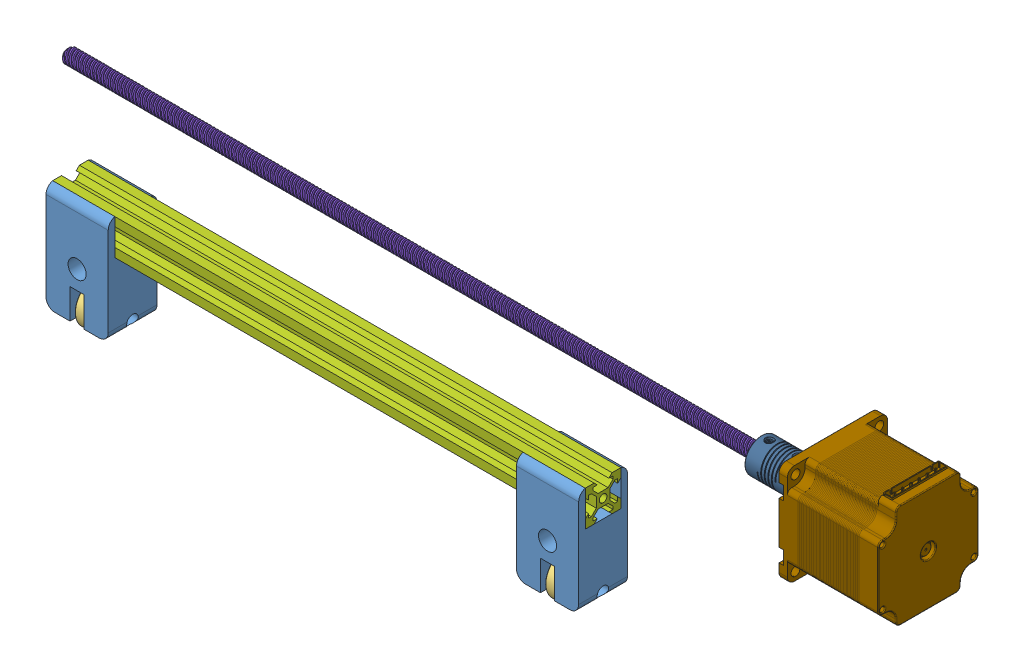
SolidWorks assembly EjeY, configuration Predeterminado. Lengths in mm.
Overall size (487.28 138.63 59).
20 component instances, 10 part files, 8 mates.
Components (placement in the parent):
- SoporteEjeY-1: SoporteEjeY [Predeterminado] at (-17.1016 3.702 20.9937) size (35 68.64 29.7)
  - SujeciónEjeY-1: SujeciónEjeY [Predeterminado] at (-24.012 20.0298 35) size (35 59.86 27.5)
  - T8-Screw-1: T8-Screw [Default] at (-6.512 2.5298 35) x (0 1 0) z (0 0 -1) size (22 22 16.4)
  - skf_bearing_61901_2-1: skf_bearing_61901_2 [Default] at (-9.4581 -20.8302 48.75) x (1 0 0) z (0 -0.067535 0.997717) size (6 24 24)
    - skf_bearing_61901_2_01-1: skf_bearing_61901_2_01 [Default] at origin size (6 24 24)
    - skf_bearing_61901_2_02-1: skf_bearing_61901_2_02 [Default] at origin size (6 16 16)
    - skf_bearing_61901_2_03-1: skf_bearing_61901_2_03 [Default] at origin size (3.18 21.18 20.29)
    - PiezaInterna-1: PiezaInterna [Predeterminado] x (0 0 -1) z (1 0 0) size (12 12 6)
- SoporteEjeY-2: SoporteEjeY [Predeterminado] at (247.6084 3.702 20.9937) size (35 68.64 29.7)
  - SujeciónEjeY-1: SujeciónEjeY [Predeterminado] at (-24.012 20.0298 35) size (35 59.86 27.5)
  - T8-Screw-1: T8-Screw [Default] at (-6.512 2.5298 35) x (0 1 0) z (0 0 -1) size (22 22 16.4)
  - skf_bearing_61901_2-1: skf_bearing_61901_2 [Default] at (-9.4581 -20.8302 48.75) x (1 0 0) z (0 -0.067535 0.997717) size (6 24 24)
    - skf_bearing_61901_2_01-1: skf_bearing_61901_2_01 [Default] at origin size (6 24 24)
    - skf_bearing_61901_2_02-1: skf_bearing_61901_2_02 [Default] at origin size (6 16 16)
    - skf_bearing_61901_2_03-1: skf_bearing_61901_2_03 [Default] at origin size (3.18 21.18 20.29)
    - PiezaInterna-1: PiezaInterna [Predeterminado] x (0 0 -1) z (1 0 0) size (12 12 6)
- BoschEjeY-1: BoschEjeY [Predeterminado] at (-41.1136 18.7318 79.7437) x (0 1 0) z (1 0 0) size (20 20 299.71)
- VarillaEjeY-1: VarillaEjeY [Default] at (339.951 77.517 52.6956) x (0 -1 0) z (1 0 0) size (8.33 8.33 405.47)
- Nema 23-1: Nema 23 [Default] at (424.5988 77.517 52.6956) x (0 0 1) z (-1 0 0) size (56.4 59.4 76.6)
- Coupler 6.35-8mm-1: Coupler 6.35-8mm [Default] at (343.2313 77.517 52.6956) x (0 0 -1) z (1 0 0) size (19.34 19.34 25)
Mates (geometry in assembly coordinates):
- Coincidente1: coincident aligned: plane of SoporteEjeY-1/SujeciónEjeY-1 through (-41.1136 23.7318 59.4937) normal (-1 0 0); plane of BoschEjeY-1 through (-41.1136 18.7318 79.7437) normal (-1 0 0)
- Coincidente2: coincident anti-aligned: plane of SoporteEjeY-1/SujeciónEjeY-1 through (-6.1136 23.7318 79.7437) normal (0 0 -1); plane of BoschEjeY-1 through (258.5964 18.7318 79.7437) normal (0 0 1)
- Coincidente3: coincident anti-aligned: plane of SoporteEjeY-1/SujeciónEjeY-1 through (-6.1136 18.7318 59.7437) normal (0 1 0); plane of BoschEjeY-1 through (258.5964 18.7318 79.7437) normal (0 -1 0)
- Coincidente4: coincident anti-aligned: plane of SoporteEjeY-2/SujeciónEjeY-1 through (258.5964 23.7318 59.7437) normal (0 0 1); plane of BoschEjeY-1 through (258.5964 18.7318 59.7437) normal (0 0 -1)
- Coincidente5: coincident aligned: plane of SoporteEjeY-2/SujeciónEjeY-1 through (258.5964 23.7318 59.4937) normal (1 0 0); plane of BoschEjeY-1 through (258.5964 18.7318 79.7437) normal (1 0 0)
- Coincidente6: coincident anti-aligned: plane of SoporteEjeY-2/SujeciónEjeY-1 through (258.5964 18.7318 59.7437) normal (0 1 0); plane of BoschEjeY-1 through (258.5964 18.7318 79.7437) normal (0 -1 0)
- Concéntrica1: concentric anti-aligned: cylinder of Nema 23-1 through (362.9988 77.517 52.6956) axis (1 0 0) radius 3.175; cylinder of Coupler 6.35-8mm-1 through (345.7313 77.517 52.6956) axis (-1 0 0) radius 4
- Concéntrica2: concentric anti-aligned: circle of VarillaEjeY-1; circle of Coupler 6.35-8mm-1
